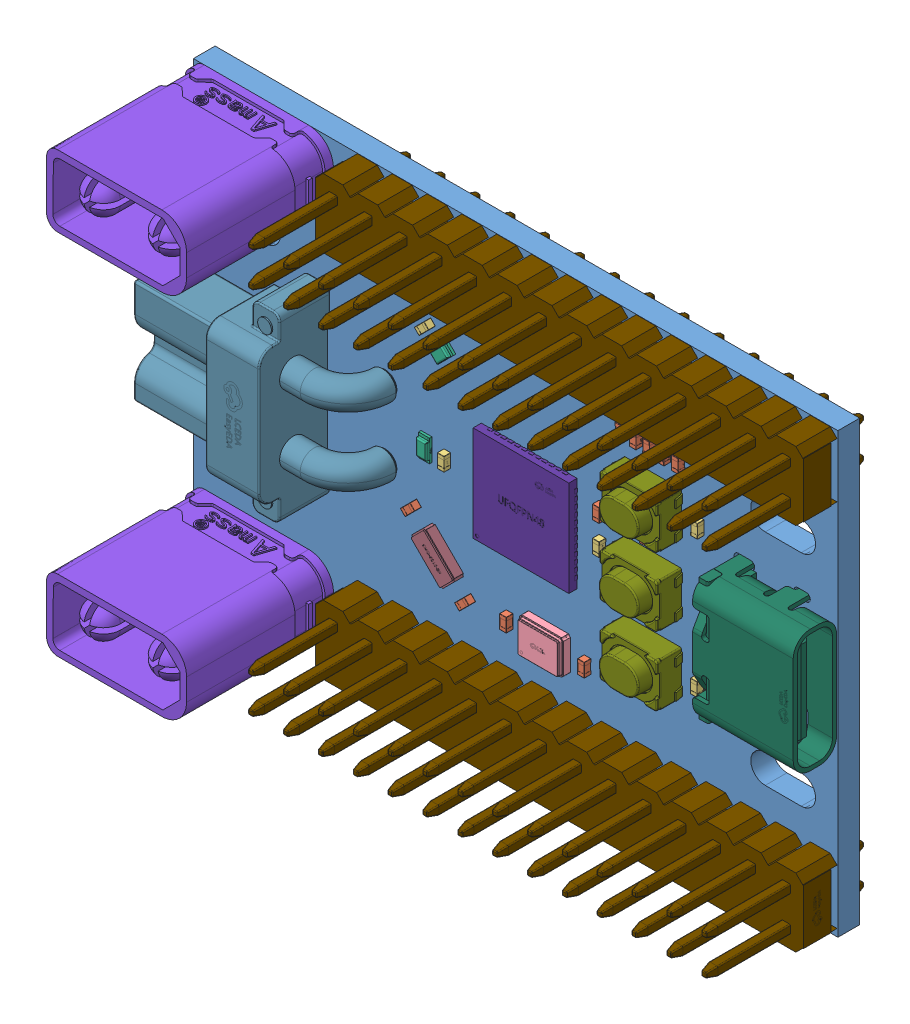
SolidWorks assembly STM32F401_BOARD_2024-09-21, configuration 默认. Lengths in mm.
Overall size (46.98 31.98 14.34).
152 component instances, 19 part files, 0 mates.
Components (placement in the parent):
- STM32F401_BOARD_2024-09-21.step-1: STM32F401_BOARD_2024-09-21.step [默认] at origin size (46.98 31.98 14.34)
  - D1.step-1: D1.step [默认] at (-1.9873 5.1919 0) x (1 0 0) z (0 0 -1) size (4.95 2.5 2.05)
    - SMA_L4.3-W2.5-LS5.0-RD.step-1: SMA_L4.3-W2.5-LS5.0-RD.step [默认] at origin size (4.95 2.5 2.05)
      - COMPOUND.step-1: COMPOUND.step [默认] at origin size (4.95 2.5 2.05)
  - C1.step-1: C1.step [默认] at (11.0937 8.4004 1.5862) x (0 -1 0) z (0 0 1) size (1 0.5 0.5)
    - C0402.step-1: C0402.step [默认] at origin size (1 0.5 0.5)
      - SOLID.step-1: SOLID.step [默认] at origin size (1 0.5 0.5)
  - C2.step-1: C2.step [默认] at (10.0526 8.4004 1.5862) x (0 -1 0) z (0 0 1) size (1 0.5 0.5)
    - C0402.step-1: C0402.step [默认] at origin size (1 0.5 0.5)
      - SOLID.step-1: SOLID.step [默认] at origin size (1 0.5 0.5)
  - C3.step-1: C3.step [默认] at (9 8.4004 1.5862) x (0 -1 0) z (0 0 1) size (1 0.5 0.5)
    - C0402.step-1: C0402.step [默认] at origin size (1 0.5 0.5)
      - SOLID.step-1: SOLID.step [默认] at origin size (1 0.5 0.5)
  - C4.step-1: C4.step [默认] at (8.0206 8.4004 1.5862) x (0 -1 0) z (0 0 1) size (1 0.5 0.5)
    - C0402.step-1: C0402.step [默认] at origin size (1 0.5 0.5)
      - SOLID.step-1: SOLID.step [默认] at origin size (1 0.5 0.5)
  - C5.step-1: C5.step [默认] at (6.985 8.4004 1.5862) x (0 -1 0) z (0 0 1) size (1 0.5 0.5)
    - C0402.step-1: C0402.step [默认] at origin size (1 0.5 0.5)
      - SOLID.step-1: SOLID.step [默认] at origin size (1 0.5 0.5)
  - C56.step-1: C56.step [默认] at (2.715 -5.745 0) x (0 -1 0) z (0 0 -1) size (1 0.5 0.5)
    - C0402.step-1: C0402.step [默认] at origin size (1 0.5 0.5)
      - SOLID.step-1: SOLID.step [默认] at origin size (1 0.5 0.5)
  - C57.step-1: C57.step [默认] at (7.874 -5.745 0) x (0 1 0) z (0 0 -1) size (1 0.5 0.5)
    - C0402.step-1: C0402.step [默认] at origin size (1 0.5 0.5)
      - SOLID.step-1: SOLID.step [默认] at origin size (1 0.5 0.5)
  - C58.step-1: C58.step [默认] at (-8.382 -4.191 1.5862) x (-0.707107 -0.707107 0) z (0 0 1) size (1 0.5 0.5)
    - C0402.step-1: C0402.step [默认] at origin size (1 0.5 0.5)
      - SOLID.step-1: SOLID.step [默认] at origin size (1 0.5 0.5)
  - C59.step-1: C59.step [默认] at (-4.4335 -8.1774 1.5862) x (-0.707107 -0.707107 0) z (0 0 1) size (1 0.5 0.5)
    - C0402.step-1: C0402.step [默认] at origin size (1 0.5 0.5)
      - SOLID.step-1: SOLID.step [默认] at origin size (1 0.5 0.5)
  - C60.step-1: C60.step [默认] at (-1.4335 -7.8898 1.5862) x (0 1 0) z (0 0 1) size (1 0.5 0.5)
    - C0402.step-1: C0402.step [默认] at origin size (1 0.5 0.5)
      - SOLID.step-1: SOLID.step [默认] at origin size (1 0.5 0.5)
  - C61.step-1: C61.step [默认] at (4.2505 -7.8898 1.5862) x (0 1 0) z (0 0 1) size (1 0.5 0.5)
    - C0402.step-1: C0402.step [默认] at origin size (1 0.5 0.5)
      - SOLID.step-1: SOLID.step [默认] at origin size (1 0.5 0.5)
  - C65.step-1: C65.step [默认] at (13.4749 -5 1.5862) x (0 -1 0) z (0 0 1) size (1 0.5 0.5)
    - C0402.step-1: C0402.step [默认] at origin size (1 0.5 0.5)
      - SOLID.step-1: SOLID.step [默认] at origin size (1 0.5 0.5)
  - C34.step-1: C34.step [默认] at (9 2.413 1.5862) x (-1 0 0) z (0 0 1) size (1 0.5 0.5)
    - C0402.step-1: C0402.step [默认] at origin size (1 0.5 0.5)
      - SOLID.step-1: SOLID.step [默认] at origin size (1 0.5 0.5)
  - C81.step-1: C81.step [默认] at (5.334 2.413 1.5862) x (0 -1 0) z (0 0 1) size (1 0.5 0.5)
    - C0402.step-1: C0402.step [默认] at origin size (1 0.5 0.5)
      - SOLID.step-1: SOLID.step [默认] at origin size (1 0.5 0.5)
  - R70.step-1: R70.step [默认] at (-7.366 7.747 1.5862) x (0.707107 0.707107 0) z (0 0 1) size (1 0.5 0.5)
    - R0402.step-1: R0402.step [默认] at origin size (1 0.5 0.5)
      - SOLID-0.step-1: SOLID-0.step [默认] at origin size (1 0.5 0.5)
  - R76.step-1: R76.step [默认] at (5.334 0.254 1.5862) x (0 -1 0) z (0 0 1) size (1 0.5 0.5)
    - R0402.step-1: R0402.step [默认] at origin size (1 0.5 0.5)
      - SOLID-0.step-1: SOLID-0.step [默认] at origin size (1 0.5 0.5)
  - R77.step-1: R77.step [默认] at (11.46 -3 0) x (-1 0 0) z (0 0 -1) size (1 0.5 0.5)
    - R0402.step-1: R0402.step [默认] at origin size (1 0.5 0.5)
      - SOLID-0.step-1: SOLID-0.step [默认] at origin size (1 0.5 0.5)
  - R78.step-1: R78.step [默认] at (11.46 3 0) x (-1 0 0) z (0 0 -1) size (1 0.5 0.5)
    - R0402.step-1: R0402.step [默认] at origin size (1 0.5 0.5)
      - SOLID-0.step-1: SOLID-0.step [默认] at origin size (1 0.5 0.5)
  - R20.step-1: R20.step [默认] at (9 -2.413 1.5862) size (1 0.5 0.5)
    - R0402.step-1: R0402.step [默认] at origin size (1 0.5 0.5)
      - SOLID-0.step-1: SOLID-0.step [默认] at origin size (1 0.5 0.5)
  - R18.step-1: R18.step [默认] at (12.5 5 1.5862) x (0 1 0) z (0 0 1) size (1 0.5 0.5)
    - R0402.step-1: R0402.step [默认] at origin size (1 0.5 0.5)
      - SOLID-0.step-1: SOLID-0.step [默认] at origin size (1 0.5 0.5)
  - R79.step-1: R79.step [默认] at (12.476 -5 1.5862) x (0 1 0) z (0 0 1) size (1 0.5 0.5)
    - R0402.step-1: R0402.step [默认] at origin size (1 0.5 0.5)
      - SOLID-0.step-1: SOLID-0.step [默认] at origin size (1 0.5 0.5)
  - R82.step-1: R82.step [默认] at (-0.4891 -3.3987 0) x (1 0 0) z (0 0 -1) size (1 0.5 0.5)
    - R0402.step-1: R0402.step [默认] at origin size (1 0.5 0.5)
      - SOLID-0.step-1: SOLID-0.step [默认] at origin size (1 0.5 0.5)
  - R83.step-1: R83.step [默认] at (-2.4736 -3.3987 0) x (1 0 0) z (0 0 -1) size (1 0.5 0.5)
    - R0402.step-1: R0402.step [默认] at origin size (1 0.5 0.5)
      - SOLID-0.step-1: SOLID-0.step [默认] at origin size (1 0.5 0.5)
  - R84.step-1: R84.step [默认] at (-5.969 0 1.5862) x (0 -1 0) z (0 0 1) size (1 0.5 0.5)
    - R0402.step-1: R0402.step [默认] at origin size (1 0.5 0.5)
      - SOLID-0.step-1: SOLID-0.step [默认] at origin size (1 0.5 0.5)
  - R85.step-1: R85.step [默认] at (-10.414 8.636 1.5862) x (-0.707107 -0.707107 0) z (0 0 1) size (1 0.5 0.5)
    - R0402.step-1: R0402.step [默认] at origin size (1 0.5 0.5)
      - SOLID-0.step-1: SOLID-0.step [默认] at origin size (1 0.5 0.5)
  - X1.step-1: X1.step [默认] at (1.4085 -7.8898 1.5862) size (3.2 2.5 0.81)
    - OSC-SMD_4P-L3.2-W2.5-BL.step-1: OSC-SMD_4P-L3.2-W2.5-BL.step [默认] at origin size (3.2 2.5 0.81)
      - SOLID-1.step-1: SOLID-1.step [默认] at origin size (3.2 2.5 0.81)
  - U8.step-1: U8.step [默认] at (-1.4049 0 0) x (0 -1 0) z (0 0 -1) size (4.9 6 1.5)
    - ESOP-8_L4.9-W3.9-P1.27-LS6.0-BL-EP-2.step-1: ESOP-8_L4.9-W3.9-P1.27-LS6.0-BL-EP-2.step [默认] at origin size (4.9 6 1.5)
      - COMPOUND-2.step-1: COMPOUND-2.step [默认] at origin size (4.9 6 1.5)
  - LED3.step-1: LED3.step [默认] at (-6.2148 6.604 1.5862) x (0.707107 0.707107 0) z (0 0 1) size (1.62 0.81 0.41)
    - LED0603-R-RD_BLUE.step-1: LED0603-R-RD_BLUE.step [默认] at origin size (1.62 0.81 0.41)
      - COMPOUND-3.step-1: COMPOUND-3.step [默认] at origin size (1.62 0.81 0.41)
  - LED4.step-1: LED4.step [默认] at (-7.493 0 1.5862) x (0 -1 0) z (0 0 1) size (1.62 0.81 0.41)
    - LED0603-R-RD_BLUE.step-1: LED0603-R-RD_BLUE.step [默认] at origin size (1.62 0.81 0.41)
      - COMPOUND-3.step-1: COMPOUND-3.step [默认] at origin size (1.62 0.81 0.41)
  - C79.step-1: C79.step [默认] at (-1.405 -5.715 0) x (-1 0 0) z (0 0 -1) size (3.7 2.8 2)
    - CASE-B_3528.step-1: CASE-B_3528.step [默认] at origin size (3.7 2.8 2)
      - COMPOUND-4.step-1: COMPOUND-4.step [默认] at origin size (3.7 2.8 2)
  - CN1.step-1: CN1.step [默认] at (-19.381 13.389 1.5862) x (-1 0 0) z (0 0 1) size (10.2 5.21 12.7)
    - CONN-TH_XT30UPB-M.step-1: CONN-TH_XT30UPB-M.step [默认] at origin size (10.2 5.21 12.7)
      - SOLID-5.step-1: SOLID-5.step [默认] at origin size (10.2 5.21 12.7)
  - CN2.step-1: CN2.step [默认] at (-19.381 -13.389 1.5862) x (-1 0 0) z (0 0 1) size (10.2 5.21 12.7)
    - CONN-TH_XT30UPB-M.step-1: CONN-TH_XT30UPB-M.step [默认] at origin size (10.2 5.21 12.7)
      - SOLID-5.step-1: SOLID-5.step [默认] at origin size (10.2 5.21 12.7)
  - U20.step-1: U20.step [默认] at (11.4603 0 0) x (0 1 0) z (0 0 -1) size (3.02 3.02 0.81)
    - TQFN-16_L3.0-W3.0-P0.50-BL-EP1.7.step-1: TQFN-16_L3.0-W3.0-P0.50-BL-EP1.7.step [默认] at origin size (3.02 3.02 0.81)
      - COMPOUND-6.step-1: COMPOUND-6.step [默认] at origin size (3.02 3.02 0.81)
  - U14.step-1: U14.step [默认] at (5.1995 -5.745 0) x (-1 0 0) z (0 0 -1) size (2.92 2.8 1.15)
    - SOT-23-5_L2.9-W1.6-P0.95-LS2.8-BL.step-1: SOT-23-5_L2.9-W1.6-P0.95-LS2.8-BL.step [默认] at origin size (2.92 2.8 1.15)
      - COMPOUND-7.step-1: COMPOUND-7.step [默认] at origin size (2.92 2.8 1.15)
  - L5.step-1: L5.step [默认] at (6.223 3.7329 0) x (0 1 0) z (0 0 -1) size (4.6 4.2 2)
    - IND-SMD_L4.6-W4.2_SMMS0420.step-1: IND-SMD_L4.6-W4.2_SMMS0420.step [默认] at origin size (4.6 4.2 2)
      - SOLID-8.step-1: SOLID-8.step [默认] at origin size (4.6 4.2 2)
  - C68.step-1: C68.step [默认] at (5.5162 -1.524 0) x (0 1 0) z (0 0 -1) size (1.6 0.8 0.8)
    - C0603.step-1: C0603.step [默认] at origin size (1.6 0.8 0.8)
      - SOLID-9.step-1: SOLID-9.step [默认] at origin size (1.6 0.8 0.8)
  - C67.step-1: C67.step [默认] at (6.9363 -1.524 0) x (0 -1 0) z (0 0 -1) size (1.6 0.8 0.8)
    - C0603.step-1: C0603.step [默认] at origin size (1.6 0.8 0.8)
      - SOLID-9.step-1: SOLID-9.step [默认] at origin size (1.6 0.8 0.8)
  - C70.step-1: C70.step [默认] at (-6.5376 0 0) x (0 1 0) z (0 0 -1) size (1.6 0.8 0.8)
    - C0603.step-1: C0603.step [默认] at origin size (1.6 0.8 0.8)
      - SOLID-9.step-1: SOLID-9.step [默认] at origin size (1.6 0.8 0.8)
  - C78.step-1: C78.step [默认] at (2.54 4.492 0) x (0 -1 0) z (0 0 -1) size (1.6 0.8 0.8)
    - C0603.step-1: C0603.step [默认] at origin size (1.6 0.8 0.8)
      - SOLID-9.step-1: SOLID-9.step [默认] at origin size (1.6 0.8 0.8)
  - C80.step-1: C80.step [默认] at (-7.9346 0 0) x (0 1 0) z (0 0 -1) size (1.6 0.8 0.8)
    - C0603.step-1: C0603.step [默认] at origin size (1.6 0.8 0.8)
      - SOLID-9.step-1: SOLID-9.step [默认] at origin size (1.6 0.8 0.8)
  - X2.step-1: X2.step [默认] at (-6.3535 -6.1604 1.5862) x (0.707107 -0.707107 0) z (0 0 1) size (3.2 1.5 0.76)
    - OSC-SMD_L3.2-W1.5.step-1: OSC-SMD_L3.2-W1.5.step [默认] at origin size (3.2 1.5 0.76)
      - COMPOUND-10.step-1: COMPOUND-10.step [默认] at origin size (3.2 1.5 0.76)
  - U31.step-1: U31.step [默认] at (-13 0 1.5862) x (0 -1 0) z (0 0 1) size (13.3 14.9 7.2)
    - CONN-TH_XT30PW-F-1.step-1: CONN-TH_XT30PW-F-1.step [默认] at origin size (13.3 14.9 7.2)
      - SOLID-11.step-1: SOLID-11.step [默认] at origin size (13.3 14.9 7.2)
  - USB1.step-1: USB1.step [默认] at (17.5011 0 1.5862) x (0 1 0) z (0 0 1) size (8.95 7.58 4.16)
    - USB-C-SMD_TYPE-C-6PIN-2MD-073.step-1: USB-C-SMD_TYPE-C-6PIN-2MD-073.step [默认] at origin size (8.95 7.58 4.16)
      - COMPOUND-12.step-1: COMPOUND-12.step [默认] at origin size (8.95 7.58 4.16)
  - SW1.step-1: SW1.step [默认] at (9 0.0072 1.5862) x (-1 0 0) z (0 0 1) size (4.7 3.2 2.51)
    - KEY-SMD_4P-L4.2-W3.2-P2.20-LS4.6.step-1: KEY-SMD_4P-L4.2-W3.2-P2.20-LS4.6.step [默认] at origin size (4.7 3.2 2.51)
      - COMPOUND-13.step-1: COMPOUND-13.step [默认] at origin size (4.7 3.2 2.51)
  - SW2.step-1: SW2.step [默认] at (9 5 1.5862) x (-1 0 0) z (0 0 1) size (4.7 3.2 2.51)
    - KEY-SMD_4P-L4.2-W3.2-P2.20-LS4.6.step-1: KEY-SMD_4P-L4.2-W3.2-P2.20-LS4.6.step [默认] at origin size (4.7 3.2 2.51)
      - COMPOUND-13.step-1: COMPOUND-13.step [默认] at origin size (4.7 3.2 2.51)
  - SW3.step-1: SW3.step [默认] at (9 -5 1.5862) x (-1 0 0) z (0 0 1) size (4.7 3.2 2.51)
    - KEY-SMD_4P-L4.2-W3.2-P2.20-LS4.6.step-1: KEY-SMD_4P-L4.2-W3.2-P2.20-LS4.6.step [默认] at origin size (4.7 3.2 2.51)
      - COMPOUND-13.step-1: COMPOUND-13.step [默认] at origin size (4.7 3.2 2.51)
  - U1.step-1: U1.step [默认] at (0 0 1.5862) size (7 7 0.61)
    - UFQFPN-48_L7.0-W7.0-P0.50-BL-EP.step-1: UFQFPN-48_L7.0-W7.0-P0.50-BL-EP.step [默认] at origin size (7 7 0.61)
      - SOLID-14.step-1: SOLID-14.step [默认] at origin size (7 7 0.61)
  - U32.step-1: U32.step [默认] at (4.6961 -13.462 1.5862) size (35.56 5 11.5)
    - HDR-TH_28P-P2.54-V-M-R2-C14-S2.54.step-1: HDR-TH_28P-P2.54-V-M-R2-C14-S2.54.step [默认] at origin size (35.56 5 11.5)
      - SOLID-15.step-1: SOLID-15.step [默认] at origin size (35.56 5 11.5)
  - U33.step-1: U33.step [默认] at (4.6961 13.462 1.5862) x (-1 0 0) z (0 0 1) size (35.56 5 11.5)
    - HDR-TH_28P-P2.54-V-M-R2-C14-S2.54.step-1: HDR-TH_28P-P2.54-V-M-R2-C14-S2.54.step [默认] at origin size (35.56 5 11.5)
      - SOLID-15.step-1: SOLID-15.step [默认] at origin size (35.56 5 11.5)
  - COMPOUND-16.step-1: COMPOUND-16.step [默认] at origin size (46.97 31.97 1.59)
